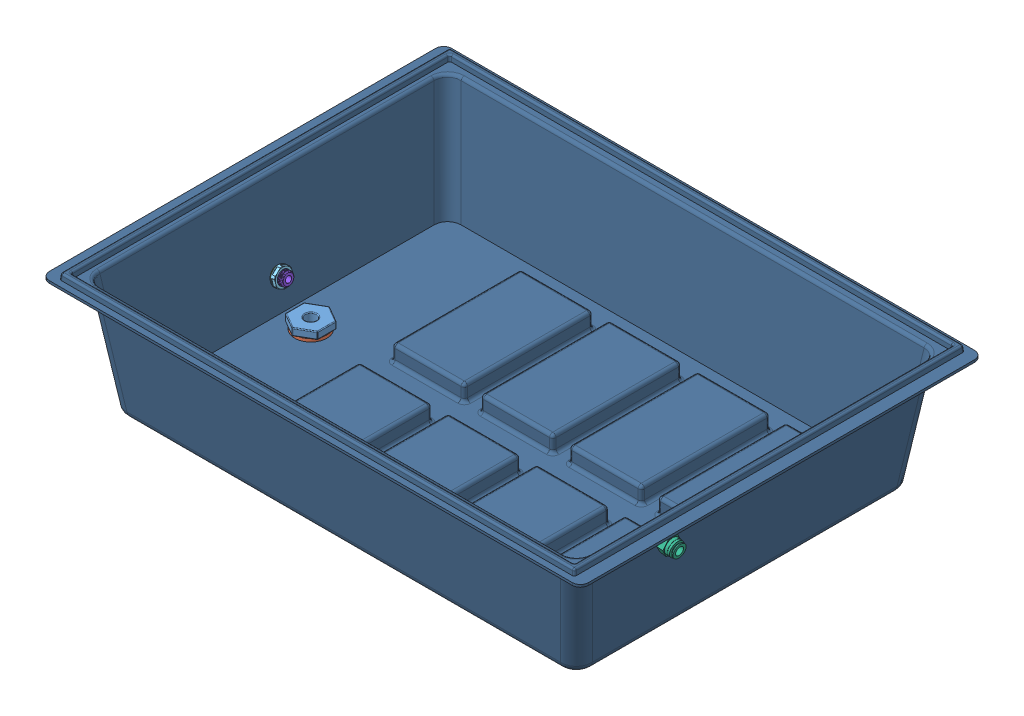
SolidWorks assembly reservroir_assembly, configuration Default. Lengths in mm.
Overall size (851.19 288.32 635).
15 component instances, 10 part files, 11 mates.
Components (placement in the parent):
- drain_assembly-1: drain_assembly [Default] at (-429.3509 -195.8779 135.5231) x (0.866025 0 0.5) z (-0.5 0 0.866025) size (58.27 70.14 50.8)
  - drain-1: drain [Default] at (3.4475 67.5493 60.8792) size (58.27 70.14 50.8)
  - drain_gasket-1: drain_gasket [Default] at (3.4475 62.9773 60.8792) size (50.8 4.57 50.8)
  - drain_nut-1: drain_nut [Default] at (3.4475 60.4373 60.8792) x (-1 0 0) z (0 0 1) size (58.11 25.4 50.8)
- TRUE_NIPPLE-1: TRUE_NIPPLE [4830K171] at (-456.8049 -187.8825 189.9698) x (0 1 0) z (0 0 1) size (28.84 22.41 22.44)
- straight_assembly-1: straight_assembly [Default] at (287.3289 37.5685 398.7278) x (0.069587 0.495134 0.866025) z (-0.990268 0.139173 0) size (37.62 36.2 41.4)
  - true_npt_nut-1: true_npt_nut [3185K112] at (-78.6901 -4.206 40.9866) size (28.95 28.95 10.31)
  - through-wall-black-1: through-wall-black [Default] at (-78.6901 -4.206 35.8304) x (0.866025 0.5 0) z (-0.5 0.866025 0) size (28.96 41.4 25.08)
  - hrd-050-gasket-1: hrd-050-gasket [Default] at (-78.6901 -4.206 40.9866) x (0.974895 0.222665 0) z (-0.222665 0.974895 0) size (25.4 2.62 25.4)
- 90_assembly-1: 90_assembly [Default] at (-497.0813 -70.7003 195.5634) x (0.017227 -0.122579 0.992309) z (0.990268 0.139173 0) size (52.61 48.36 69.22)
  - true_npt_nut-1: true_npt_nut [3185K112] at (-3.8428 13.2999 -10.4025) size (28.95 28.95 10.31)
  - hrd-050-gasket-1: hrd-050-gasket [Default] at (-3.8428 13.2999 -13.0187) x (0.930255 -0.366913 0) z (-0.366913 -0.930255 0) size (25.4 2.62 25.4)
  - through-wall-90-1: through-wall-90 [Default] at (-3.8428 13.2999 -15.5587) x (-0.797473 0.603354 0) z (-0.603354 -0.797473 0) size (46.99 69.22 25.08)
- threaded_threaded_90-1: threaded_threaded_90 [Default] at (-425.0549 -220.7665 189.9698) x (0 -1 0) z (1 0 0) size (46.22 27.78 46.59)
- GMR.505-1: GMR.505 [Default] at (-139.0726 40.4544 190.1039) size (850.9 190.37 635)
Mates (geometry in assembly coordinates):
- Concentric2: concentric: circle of drain_assembly-1/drain-1; cylinder of TRUE_NIPPLE-1 through (-456.8049 -202.3018 189.9698) axis (0 1 0) radius 7.8994
- Coincident3: coincident: plane of drain_assembly-1/drain-1 through (-456.8049 -186.7486 189.9698) normal (0 -1 0); circle of TRUE_NIPPLE-1
- Parallel4: parallel: plane of drain_assembly-1/drain-1 through (-456.8049 -186.7486 189.9698) normal (0 -1 0); plane of threaded_threaded_90-1 through (-456.8049 -189.0165 189.9698) normal (0 1 0)
- Concentric5: concentric: circle of drain_assembly-1/drain-1; circle of threaded_threaded_90-1
- Coincident8: coincident: plane of TRUE_NIPPLE-1 through (-456.8049 -189.0165 189.9698) normal (0 -1 0); plane of threaded_threaded_90-1 through (-456.8049 -189.0165 189.9698) normal (0 1 0)
- Concentric6: concentric: cylinder of 90_assembly-1/true_npt_nut-1 through (-505.612 -220.2725 190.1039) axis (0.990268 0.139173 0) radius 14.4759; cylinder of GMR.505-1 through (-570.5444 -229.3982 190.1039) axis (0.990268 0.139173 0) radius 11.1125
- Coincident9: coincident: plane of 90_assembly-1/hrd-050-gasket-1 through (-508.2028 -220.6366 190.1039) normal (-0.990268 -0.139173 0); plane of GMR.505-1 through (-526.4597 -90.7317 -99.4561) normal (0.990268 0.139173 0)
- Concentric7: concentric: cylinder of straight_assembly-1/through-wall-black-1 through (255.9256 -136.9544 332.6832) axis (-0.990268 0.139173 0) radius 11.811; cylinder of GMR.505-1 through (-556.2249 -22.8141 332.6832) axis (0.990268 -0.139173 0) radius 11.1125
- Coincident10: coincident: plane of straight_assembly-1/through-wall-black-1 through (245.8644 -135.5404 332.6832) normal (-0.990268 0.139173 0); plane of GMR.505-1 through (252.0874 -91.262 479.6639) normal (0.990268 -0.139173 0)
- Concentric8: concentric: cylinder of drain_assembly-1/drain_gasket-1 through (-456.5726 -128.3286 190.1039) axis (0 -1 0) radius 25.4; cylinder of GMR.505-1 through (-456.5726 -136.7106 190.1039) axis (0 1 0) radius 19.05
- Coincident11: coincident: plane of drain_assembly-1/drain_gasket-1 through (-456.5726 -132.9006 190.1039) normal (0 -1 0); plane of GMR.505-1 through (-139.0726 -132.9006 190.1039) normal (0 1 0)
